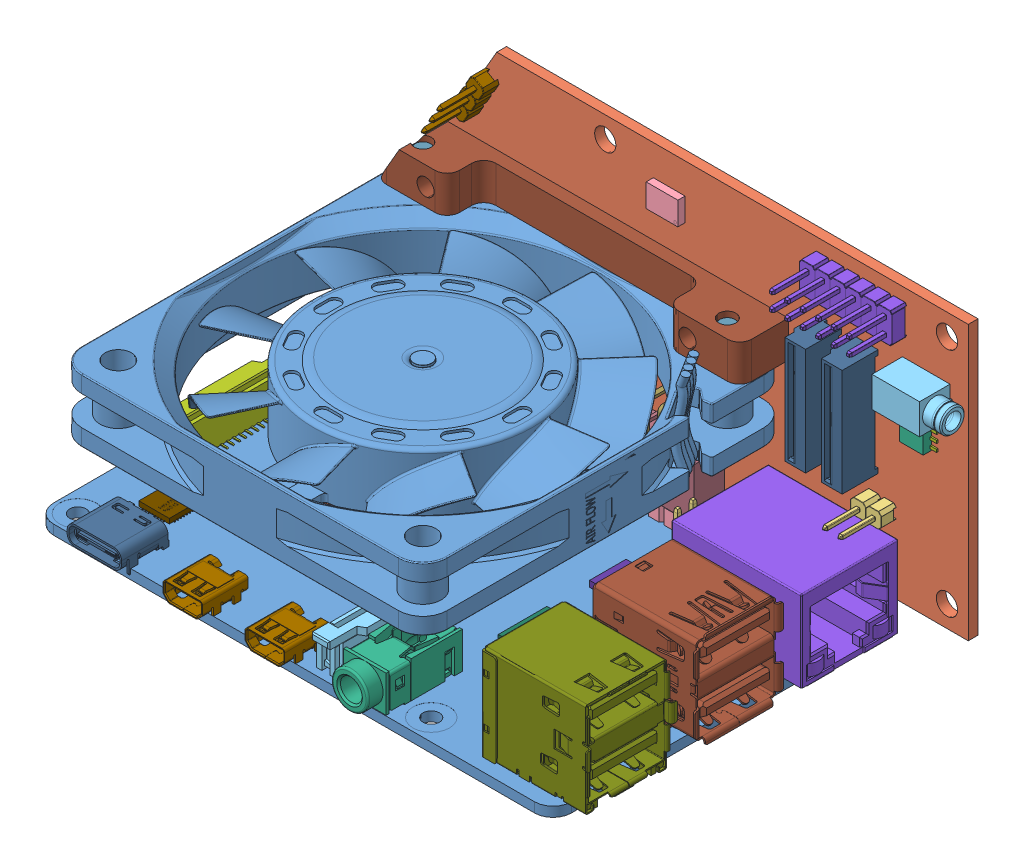
SolidWorks assembly Raspberry Pi Module, configuration Default. Lengths in mm.
Overall size (98.2 52.2 64.29).
53 component instances, 33 part files, 21 mates.
Components (placement in the parent):
- Raspberry Pi 4 Model B-1: Raspberry Pi 4 Model B [Default] at origin size (88.99 19.9 58.4)
  - PCB, RPi4ModelB-1: PCB, RPi4ModelB [Default] at origin size (85 1.6 56)
  - Broadcom BCM2711B0 CPU, RPi4ModelB-1: Broadcom BCM2711B0 CPU, RPi4ModelB [Default] at (-13.25 0.8 -4.5) size (15 2.3 15)
  - 2.54 mm DUPONT MALE PIN HEADER, POE, 2X2, RPi4ModelB-1: 2.54 mm DUPONT MALE PIN HEADER, POE, 2X2, RPi4ModelB [Default] at (19 0.8 -18.5) size (5.08 11.3 5.08)
  - 2.54 mm DUPONT MALE PIN HEADER, IO, 2X20, RPi4ModelB-1: 2.54 mm DUPONT MALE PIN HEADER, IO, 2X20, RPi4ModelB [Default] at (-10 0.8 -24.5) size (50.8 11.3 5.08)
  - Camera Connector, RPi4ModelB-1: Camera Connector, RPi4ModelB [Default] at (4 0.8 16.5) x (0 0 -1) z (1 0 0) size (22.4 5.68 5.07)
  - Microphone Plug, RPi4ModelB-1: Microphone Plug, RPi4ModelB [Default] at (11.5 0.8 21.65) size (7.23 7.55 15)
  - Display Connector, RPi4ModelB-1: Display Connector, RPi4ModelB [Default] at (-38.5 0.8 0) x (0 0 1) z (-1 0 0) size (22.4 5.68 5.07)
  - Gigabit Ethernet Port, RPi4ModelB-1: Gigabit Ethernet Port, RPi4ModelB [Default] at (45.5 7.55 -17.75) x (0 0 -1) z (1 0 0) size (16.2 17.24 21.64)
  - Female Micro HDMI Connector, RPi4ModelB-2: Female Micro HDMI Connector, RPi4ModelB [Default] at (-3 0.8 27.3875) size (6.5 3.51 7.5)
  - Female Micro HDMI Connector, RPi4ModelB-3: Female Micro HDMI Connector, RPi4ModelB [Default] at (-16.5 0.8 27.3875) size (6.5 3.51 7.5)
  - Female USB Type C Connector, RPi4ModelB-1: Female USB Type C Connector, RPi4ModelB [Default] at (-31.3 0.8 26.5419) size (8.94 3.96 7.9)
  - 2X USB3.0 PORTS, RPi4ModelB-2: 2X USB3.0 PORTS, RPi4ModelB [Default] at (37.07 0.8 1) size (17.47 19.41 15.68)
  - 91D77 D9WHV 778K, 4 GB LPDDR4 SDRAM, RPi4ModelB-1: 91D77 D9WHV 778K, 4 GB LPDDR4 SDRAM, RPi4ModelB [Default] at (2.25 0.8 -4.5) size (10 0.8 14.5)
  - Cypress CYW43455 Wireless Module Cover, RPi4ModelB-1: Cypress CYW43455 Wireless Module Cover, RPi4ModelB [Default] at (-30.5 0.8 -14.5) size (11 1.6 13)
  - SD Card Slot, RPi4ModelB-1: SD Card Slot, RPi4ModelB [Default] at (-35.3 -0.8 0) x (0 0 -1) z (-1 0 0) size (11.95 1.45 11.4)
  - VIA VL805 PCIe USB 3.0 controller, RPi4ModelB-1: VIA VL805 PCIe USB 3.0 controller, RPi4ModelB [Default] at (17.5 0.8 4) size (8.8 0.8 8.8)
  - 2X USB2.0 PORTS, RPi4ModelB-1: 2X USB2.0 PORTS, RPi4ModelB [Default] at (37.065 0.65 19) size (17.87 19.16 15.33)
  - Broadcom BCM54213PE Gigabit Ethernet Transceiver, RPi4ModelB-1: Broadcom BCM54213PE Gigabit Ethernet Transceiver, RPi4ModelB [Default] at (16.5 0.8 -10) size (6.8 1 6.8)
  - MxL7704 Universal PMIC, RPi4ModelB-1: MxL7704 Universal PMIC, RPi4ModelB [Default] at (-32.5 0.8 16) size (5.4 0.8 5.4)
- FAN 6010-1: FAN 6010 [Default] at (-3.85 19.0762 3.0235) x (-1 0 0) z (0 1 0) size (62.48 62.48 15.97)
- Extension Board-1: Extension Board [Default] at (6.598 25.3 -28.5765) x (-1 0 0) z (0 0 1) size (98.2 45 11.69)
  - Extension PCB-1: Extension PCB [Default] at origin size (98.2 45 1.6)
  - 2302-6111-TG 5,84.STEP-1: 2302-6111-TG 5,84.STEP [Default] at (-33.568 8.8346 1.6) x (-1 0 0) z (0 1 0) size (5.08 10.93 2.54)
    - 2302-6111-TG.STEP-1: 2302-6111-TG.STEP [Default] at origin size (2.54 10.93 2.54)
    - 2302-6111-TG.STEP-2: 2302-6111-TG.STEP [Default] at (2.54 0 0) size (2.54 10.93 2.54)
  - BNO080--3DModel-STEP-56544.step-1: BNO080--3DModel-STEP-56544.step [Default] at (0 -17.1 1.6) x (1 0 0) z (0 -1 0) size (5.2 1.18 3.8)
  - CUI_DEVICES_SJ1-2503A-1: CUI_DEVICES_SJ1-2503A [Default] at (-49.098 -11.5 4.1) x (-1 0 0) z (0 1 0) size (11.15 7.5 5)
  - MIX3022-1: MIX3022 [Default] at (-41.148 -5.55 1.6) x (0 -1 0) z (0 0 1) size (4.9 6 1.4)
    - MIX3022 Body-1: MIX3022 Body [Default] at origin size (4.9 3.9 1.4)
    - MIX3022 Contact-1: MIX3022 Contact [Default] at (-1.905 2.475 0) size (0.45 1.05 0.25)
    - MIX3022 Contact-2: MIX3022 Contact [Default] at (-0.635 2.475 0) size (0.45 1.05 0.25)
    - MIX3022 Contact-3: MIX3022 Contact [Default] at (0.635 2.475 0) size (0.45 1.05 0.25)
    - MIX3022 Contact-4: MIX3022 Contact [Default] at (1.905 2.475 0) size (0.45 1.05 0.25)
    - MIX3022 Contact-5: MIX3022 Contact [Default] at (-1.905 -2.475 0) x (-1 0 0) z (0 0 1) size (0.45 1.05 0.25)
    - MIX3022 Contact-6: MIX3022 Contact [Default] at (-0.635 -2.475 0) x (-1 0 0) z (0 0 1) size (0.45 1.05 0.25)
    - MIX3022 Contact-7: MIX3022 Contact [Default] at (0.635 -2.475 0) x (-1 0 0) z (0 0 1) size (0.45 1.05 0.25)
    - MIX3022 Contact-8: MIX3022 Contact [Default] at (1.905 -2.475 0) x (-1 0 0) z (0 0 1) size (0.45 1.05 0.25)
  - PH2-12-UA.step-1: PH2-12-UA.step [Default] at (-25.128 -19.5 2.85) x (1 0 0) z (0 -1 0) size (15.24 11.55 5)
  - PR20C03VBDN.STEP-1: PR20C03VBDN.STEP [Default] at (29.5268 -19.5674 1.6) x (0.5 0.866025 0) z (0.866025 -0.5 0) size (7.62 11.64 2.54)
    - PR20203VBNN.STEP-1: PR20203VBNN.STEP [Default] at origin size (2.54 11.64 2.54)
    - PR20203VBNN.STEP-2: PR20203VBNN.STEP [Default] at (2.54 0 0) size (2.54 11.64 2.54)
    - PR20203VBNN.STEP-3: PR20203VBNN.STEP [Default] at (5.08 0 0) size (2.54 11.64 2.54)
  - 15pin flex 1mm th.stp-1: 15pin flex 1mm th.stp [Default] at (-26.348 -12.7 4.55) x (0 -1 0) z (0 0 1) size (17.6 3.9 8.93)
  - 15pin flex 1mm th.stp-2: 15pin flex 1mm th.stp [Default] at (-32.348 -12.7 4.55) x (0 -1 0) z (0 0 1) size (17.6 3.9 8.93)
- Fan mount-2: Fan mount [Default] at (-3.85 32.4262 -26.9765) size (59.34 6 8)
- 2x20 100mil female header ra-1: 2x20 100mil female header ra [Default] at (-10 11.809 -24.5) x (1 0 0) z (0 0 -1) size (51.31 12.78 7.48)
  - SSW_120_02_T_D_RA_3-1: SSW_120_02_T_D_RA_3 [Default] at (0 -1.7272 0) size (49.3 5.28 6.88)
  - SSW_120_02_T_D_RA_5-1: SSW_120_02_T_D_RA_5 [Default] at origin size (51.31 8.51 4.95)
- Metric button hex socket screw-1: Metric button hex socket screw [ISO 7380 - M3 x 16 --- 16C] at (21.15 16.9762 -21.9765) x (0 1 0) z (0.090126 0 -0.99593) size (17.65 5.7 5.7)
- Metric button hex socket screw-2: Metric button hex socket screw [ISO 7380 - M3 x 16 --- 16C] at (-28.85 16.9762 -21.9765) x (0 1 0) z (-0.451554 0 0.892244) size (17.65 5.7 5.7)
- Metric Washer-1: Metric Washer [M3.5 WASHER] at (21.15 19.0762 -21.9765) x (-1 0 0) z (0 -1 0) size (8 8 0.45)
- Metric Washer-2: Metric Washer [M3 WASHER] at (-28.85 19.0762 -21.9765) x (1 0 0) z (0 -1 0) size (7 7 0.45)
Mates (geometry in assembly coordinates):
- Coincident7: coincident anti-aligned: plane of FAN 6010-1 through (-29.85 19.0762 -26.9765) normal (0 0 -1); plane of Extension Board-1/Extension PCB-1 through (6.598 25.3 -26.9765) normal (0 0 1)
- Distance6: distance = 2 mm anti-aligned: plane of Raspberry Pi 4 Model B-1/Gigabit Ethernet Port, RPi4ModelB-1 through (24.15 7.55 -17.75) normal (-1 0 0); plane of FAN 6010-1 through (26.15 19.0762 -22.9765) normal (1 0 0)
- Coincident11: coincident anti-aligned: plane of 2x20 100mil female header ra-1/SSW_120_02_T_D_RA_5-1 through (-35.654 3.3 -26.9765) normal (0 0 -1); plane of Extension Board-1/Extension PCB-1 through (6.598 25.3 -26.9765) normal (0 0 1)
- Distance2: distance = 7 mm: plane of 2x20 100mil female header ra-1/SSW_120_02_T_D_RA_5-1 through (-10 3.3 -24.5) normal (0 -1 0); line of Extension Board-1/Extension PCB-1 through (55.696 10.3 -28.5765) axis (-1 0 0)
- Distance4: distance = 25 mm: plane of Raspberry Pi Extension Board-1/Raspberry Pi Extension PCB-1 through (55.696 10.3 -26.9765) normal (1 0 0); plane of SSW_120_02_T_D_RA-1/SSW_120_02_T_D_RA_5-1 through (15.654 3.3 -26.9765) normal (1 0 0)
- Coincident12: coincident anti-aligned: plane of Raspberry Pi 4 Model B-1/2.54 mm DUPONT MALE PIN HEADER, IO, 2X20, RPi4ModelB-1 through (-34.13 3.3 -25.77) normal (0 1 0); plane of 2x20 100mil female header ra-1/SSW_120_02_T_D_RA_5-1 through (-10 3.3 -24.5) normal (0 -1 0)
- Concentric2: concentric anti-aligned: circle of Raspberry Pi 4 Model B-1/2.54 mm DUPONT MALE PIN HEADER, IO, 2X20, RPi4ModelB-1; circle of SSW_120_02_T_D_RA-1/SSW_120_02_T_D_RA_5-1
- Parallel2: parallel anti-aligned: plane of Raspberry Pi 4 Model B-1/PCB, RPi4ModelB-1 through (-42.5 0.8 -28) normal (0 0 -1); plane of 2x20 100mil female header ra-1/SSW_120_02_T_D_RA_5-1 through (15.654 3.3 -22.0235) normal (0 0 1)
- Distance5: distance = 3 mm anti-aligned: plane of FAN 6010-1 through (-3.85 19.0762 3.0235) normal (0 -1 0); plane of 2x20 100mil female header ra-1/SSW_120_02_T_D_RA_3-1 through (14.6507 16.0762 -29.5038) normal (0 1 0)
- Coincident13: coincident aligned: plane of Raspberry Pi 4 Model B-1/PCB, RPi4ModelB-1 through (-42.5 0.8 -28) normal (-1 0 0); plane of Extension Board-1/Extension PCB-1 through (-42.5 4.3 -26.9765) normal (-1 0 0)
- Coincident15: coincident aligned: plane of Extension Board-1/Extension PCB-1 through (6.598 25.3 -26.9765) normal (0 0 1); plane of Fan mount-2 through (-3.85 32.4262 -26.9765) normal (0 0 1)
- Coincident17: coincident anti-aligned: plane of FAN 6010-1 through (-3.85 19.0762 3.0235) normal (-1 0 0); plane of Fan mount-2 through (-3.85 32.4262 -26.9765) normal (1 0 0)
- Coincident18: coincident anti-aligned: plane of FAN 6010-1 through (-3.85 29.4262 3.0235) normal (0 1 0); plane of Fan mount-2 through (-33.85 29.4262 -24.9765) normal (0 -1 0)
- Concentric16807135734: concentric anti-aligned: cylinder of FAN 6010-1 through (21.15 19.0762 -21.9765) axis (0 1 0) radius 2.15; cylinder of Metric button hex socket screw-1 through (21.15 16.9762 -21.9765) axis (0 -1 0) radius 2.85
- Coincident2820729582: coincident anti-aligned: plane of Metric Washer-1 through (21.15 18.6262 -21.9765) normal (0 -1 0); plane of Metric button hex socket screw-1 through (22.6439 18.6262 -21.8413) normal (0 1 0)
- Concentric16807135744: concentric anti-aligned: cylinder of FAN 6010-1 through (-28.85 19.0762 -21.9765) axis (0 1 0) radius 2.15; cylinder of Metric button hex socket screw-2 through (-28.85 16.9762 -21.9765) axis (0 -1 0) radius 2.85
- Coincident2820729592: coincident anti-aligned: plane of Metric Washer-2 through (-28.85 18.6262 -21.9765) normal (0 -1 0); plane of Metric button hex socket screw-2 through (-30.1884 18.6262 -22.6538) normal (0 1 0)
- Concentric31: concentric anti-aligned: cylinder of Metric Washer-1 through (21.15 18.6262 -21.9765) axis (0 1 0) radius 1.85; circle of Metric button hex socket screw-1
- Coincident191: coincident anti-aligned: plane of FAN 6010-1 through (-3.85 19.0762 3.0235) normal (0 -1 0); plane of Metric Washer-1 through (21.15 19.0762 -21.9765) normal (0 1 0)
- Concentric41: concentric anti-aligned: cylinder of Metric Washer-2 through (-28.85 18.6262 -21.9765) axis (0 1 0) radius 1.6; circle of Metric button hex socket screw-2
- Coincident201: coincident anti-aligned: plane of FAN 6010-1 through (-3.85 19.0762 3.0235) normal (0 -1 0); plane of Metric Washer-2 through (-28.85 19.0762 -21.9765) normal (0 1 0)
